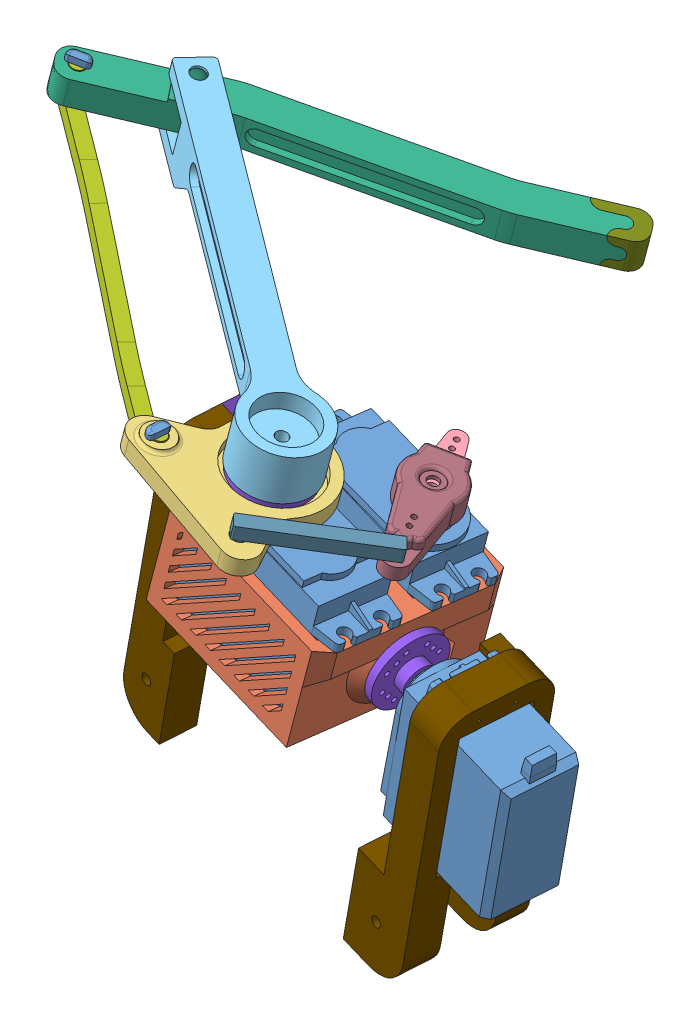
SolidWorks assembly Rear Robot Assembly, configuration Default. Lengths in mm.
Overall size (187.45 151.33 155.87).
34 component instances, 19 part files, 63 mates.
Components (placement in the parent):
- MG996R-1: MG996R [Default] at (29.5952 -122.5628 58.2658) x (-0.962615 0.249609 -0.105199) z (0.100626 -0.031047 -0.99444) size (54.5 42.75 20)
- MG996R-2: MG996R [Default] at (26.9789 -121.7556 84.1213) x (0.962615 -0.249609 0.105199) z (-0.100626 0.031047 0.99444) size (54.5 42.75 20)
- MG996R-3: MG996R [Default] at (100.7498 -138.2322 78.1733) x (-0.241344 -0.966685 -0.085287) z (0.122983 0.056709 -0.990787) size (54.5 42.75 20)
- Servo Housing-1: Servo Housing [Default] at (37.077 -93.7693 58.1239) x (-0.962615 0.249609 -0.105199) z (0.251487 0.967849 -0.00477) size (61.5 52 29.25)
- Rotating Piece-1: Rotating Piece [Default] at (26.8579 -80.6595 82.9278) x (0.452738 -0.121993 -0.883259) z (0.855443 -0.219969 0.468862) size (44.28 6 43.21)
- Double_Blade_Rudder-1: Double_Blade_Rudder [默认] at (51.0424 -81.5852 59.0548) x (0.86578 -0.227163 -0.445894) z (-0.432642 0.108008 -0.895073) size (12.2 5.5 38)
- Upper Leg-1: Upper Leg [Default] at (-58.4119 -49.1581 29.3225) x (-0.531201 0.142144 0.835237) z (0.251487 0.967849 -0.00477) size (22 116.4 18)
- Lower leg-1: Lower leg [Default] at (34.7159 -67.9253 -21.6894) x (0.593284 -0.150263 0.790845) z (-0.251487 -0.967849 0.00477) size (20.21 126 9.59)
- Long Connection Rod-1: Long Connection Rod [Default] at (10.1683 -76.252 97.3115) x (0.530048 -0.141848 -0.836019) z (-0.809817 0.20772 -0.548679) size (5 22 105.4)
- Circle Rudder-1: Circle Rudder [默认] at (57.8128 -116.2822 73.9977) x (0.107242 0.707834 0.698191) z (0.248738 0.660808 -0.70814) size (20.8 5.5 20.8)
- 688ZZ Bearing Assembly-2: 688ZZ Bearing Assembly [Default] at (1.0185 -101.5553 67.791) x (-0.264501 -0.949925 0.166376) z (-0.962615 0.249609 -0.105199) size (17.99 17.98 5)
  - Outer Ring-1: Outer Ring [Default] at origin size (16 16 5)
  - Inner Ring-1: Inner Ring [Default] x (-0.241565 -0.970385 0) z (0 0 1) size (10.6 10.6 5)
  - Cage-1: Cage [Default] x (0.535517 0.844524 0) z (0 0 1) size (13.01 13.06 2.21)
  - 2mm Ball Bearing-1: 2mm Ball Bearing [Default] at (-5.0671 3.2131 0) x (0.050652 0.835774 0.546732) z (0.977207 -0.154478 0.145614) size (2 2 2)
  - 2mm Ball Bearing-2: 2mm Ball Bearing [Default] at (-5.988 -0.3789 0) x (-0.450278 0.705928 0.546732) z (0.881377 0.449412 0.145614) size (2 2 2)
  - 2mm Ball Bearing-3: 2mm Ball Bearing [Default] at (-4.6217 -3.8262 0) x (-0.779216 0.306441 0.546732) z (0.448891 0.881642 0.145614) size (2 2 2)
  - 2mm Ball Bearing-4: 2mm Ball Bearing [Default] at (-1.49 -5.812 0) x (-0.810521 -0.210096 0.546732) z (-0.155056 0.977115 0.145614) size (2 2 2)
  - 2mm Ball Bearing-5: 2mm Ball Bearing [Default] at (2.2108 -5.5778 0) x (-0.532234 -0.646383 0.546732) z (-0.699777 0.699363 0.145614) size (2 2 2)
  - 2mm Ball Bearing-6: 2mm Ball Bearing [Default] at (5.0671 -3.2131 0) x (-0.050652 -0.835774 0.546732) z (-0.977207 0.154478 0.145614) size (2 2 2)
  - 2mm Ball Bearing-7: 2mm Ball Bearing [Default] at (5.988 0.3789 0) x (0.450278 -0.705928 0.546732) z (-0.881377 -0.449412 0.145614) size (2 2 2)
  - 2mm Ball Bearing-8: 2mm Ball Bearing [Default] at (4.6217 3.8262 0) x (0.779216 -0.306441 0.546732) z (-0.448891 -0.881642 0.145614) size (2 2 2)
  - 2mm Ball Bearing-9: 2mm Ball Bearing [Default] at (1.49 5.812 0) x (0.810521 0.210096 0.546732) z (0.155056 -0.977115 0.145614) size (2 2 2)
  - 2mm Ball Bearing-10: 2mm Ball Bearing [Default] at (-2.2108 5.5778 0) x (0.532234 0.646383 0.546732) z (0.699777 -0.699363 0.145614) size (2 2 2)
- Circle Rudder-3: Circle Rudder [默认] at (28.1908 -75.5299 82.9026) x (0.821577 -0.21087 0.529666) z (0.511631 -0.137123 -0.848193) size (20.8 5.5 20.8)
- Servo Arm Mount-1: Servo Arm Mount [Default] at (51.0424 -81.5852 59.0548) x (-0.86578 0.227163 0.445894) z (0.251487 0.967849 -0.00477) size (16.2 34.39 7.06)
- Short Connecting Rod-1: Short Connecting Rod [Default] at (63.207 -84.6449 79.6012) x (-0.679733 0.180127 0.710998) z (0.251487 0.967849 -0.00477) size (37.08 4 13)
- 91595A167_Dowel Pin-1: 91595A167_Dowel Pin [91595A167] at (-52.0367 -50.8228 27.674) x (-0.945505 0.244623 -0.214897) z (-0.251487 -0.967849 0.00477) size (4 4 20)
- Foot Cap-1: Foot Cap [Default] at (18.0805 -63.5858 -21.0299) x (0.593284 -0.150263 0.790845) z (-0.251487 -0.967849 0.00477) size (10.5 14 9.53)
- Lower Leg Mount-1: Lower Leg Mount [Default] at (-1.6759 -81.5579 68.6011) x (0.241344 0.966685 0.085287) z (0.962615 -0.249609 0.105199) size (41.75 15.4 10)
- Reverse Side Leg Mount-1: Reverse Side Leg Mount [Default] at (-136.4701 -136.4866 64.2689) x (0.241344 0.966685 0.085287) z (0.962615 -0.249609 0.105199) size (86 33.8 96.5)
- Rod Cap-1: Rod Cap [Default] at (-70.679 -41.0418 44.0662) x (-0.863943 0.226704 0.449674) z (0.436298 -0.108967 0.89318) size (6.08 7 3)
- Rod Cap-2: Rod Cap [Default] at (9.6296 -69.6975 99.0476) x (-0.054126 0.018984 0.998354) z (0.966346 -0.250815 0.05716) size (6.08 7 3)
- Rod Cap-3: Rod Cap [Default] at (35.666 -82.9502 103.5021) x (-0.679733 0.180127 0.710998) z (-0.688997 0.175565 -0.703178) size (6.08 7 3)
Mates (geometry in assembly coordinates):
- Coincident3: coincident aligned: plane of MG996R-1 through (49.2065 -88.6505 59.0896) normal (0.251487 0.967849 -0.00477); plane of MG996R-2 through (26.3549 -82.5952 82.9374) normal (0.251487 0.967849 -0.00477)
- Coincident4: coincident aligned: plane of MG996R-1 through (59.0851 -93.3273 50.2812) normal (0.962615 -0.249609 0.105199); plane of MG996R-2 through (54.4563 -91.8991 96.0254) normal (0.962615 -0.249609 0.105199)
- Distance1: distance = 6 mm anti-aligned: plane of MG996R-1 through (57.0726 -92.7063 70.17) normal (-0.100626 0.031047 0.99444); plane of MG996R-2 through (17.4829 -82.4109 71.8761) normal (0.100626 -0.031047 -0.99444)
- InPlace1: in place: plane of ? through (-38.4551 28.1284 17.4765) normal (0 1 0); plane of ? through (0 28.1284 0) normal (0 1 0); moOrthogonalPlaneRef_w of ? through (-38.4551 28.1284 17.4765) normal (0 1 0); plane of ? through (0 28.1284 0) normal (0 0 -1); plane of ? through (-38.4551 28.1284 17.4765) normal (0 1 0); plane of ? through (0 28.1284 0) normal (1 0 0); plane of MG996R-1 through (12.5314 -87.3809 60.2393) normal (0.251487 0.967849 -0.00477); unknown of Servo Housing-1
- Coincident6: coincident aligned: plane of MG996R-1; plane of Servo Housing-1
- Coincident7: coincident aligned: moOrthogonalPlaneRef_w of MG996R-1; plane of Servo Housing-1 through (37.077 -93.7693 58.1239) normal (-0.100626 0.031047 0.99444)
- Coincident8: coincident anti-aligned: moOrthogonalPlaneRef_w of MG996R-1; plane of Servo Housing-1 through (37.077 -93.7693 58.1239) normal (-0.962615 0.249609 -0.105199)
- Concentric1: concentric aligned: cylinder of MG996R-1 through (49.7095 -86.7148 59.0801) axis (0.251487 0.967849 -0.00477) radius 1.5; circle of Rotating Piece-1
- Coincident5: coincident anti-aligned: plane of MG996R-1 through (49.7095 -86.7148 59.0801) normal (0.251487 0.967849 -0.00477); plane of Rotating Piece-1 through (26.8579 -80.6595 82.9278) normal (-0.251487 -0.967849 0.00477)
- Coincident7: coincident anti-aligned: plane of MG996R-2 through (27.6124 -77.756 82.9135) normal (0.251487 0.967849 -0.00477); plane of Double_Blade_Rudder-1 through (50.4639 -83.8113 59.0657) normal (-0.251487 -0.967849 0.00477)
- Concentric2: concentric aligned: cylinder of MG996R-2 through (13.057 -90.8527 63.064) axis (0.25828 0.962853 -0.078774) radius 1.5; cylinder of Double_Blade_Rudder-1 through (36.5135 23.7673 6.6118) axis (0.25828 0.962853 -0.078774) radius 1.5
- Concentric3: concentric aligned: cylinder of Rotating Piece-1 through (27.3609 -78.7238 82.9183) axis (-0.251487 -0.967849 0.00477) radius 4.75; cylinder of Upper Leg-1 through (30.4542 -66.8193 82.8596) axis (-0.251487 -0.967849 0.00477) radius 1.5
- Concentric4: concentric aligned: cylinder of Upper Leg-1 through (-54.0486 -58.5656 27.7121) axis (0.251487 0.967849 -0.00477) radius 2.1; cylinder of Lower leg-1 through (-52.9169 -54.2102 27.6907) axis (0.251487 0.967849 -0.00477) radius 2
- Distance3: distance = 0.5 mm anti-aligned: plane of Lower leg-1 through (34.7159 -67.9253 -21.6894) normal (0.251487 0.967849 -0.00477); plane of Upper Leg-1 through (-48.4038 -45.6253 15.9301) normal (-0.251487 -0.967849 0.00477)
- LimitAngle3: limit planar angle = 1.561857 rad anti-aligned: plane of Lower leg-1 through (32.4525 -76.6359 -21.6465) normal (0.593284 -0.150263 0.790845); plane of Upper Leg-1 through (-50.585 -40.9011 20.9224) normal (0.531201 -0.142144 -0.835237)
- Coincident16: coincident anti-aligned: plane of Long Connection Rod-1 through (10.1683 -76.252 97.3115) normal (0.251487 0.967849 -0.00477); plane of Rotating Piece-1 through (26.8579 -80.6595 82.9278) normal (-0.251487 -0.967849 0.00477)
- Concentric9: concentric anti-aligned: cylinder of Lower leg-1 through (-47.0306 -55.7879 17.9084) axis (0.251487 0.967849 -0.00477) radius 2.1; cylinder of Connection Rod (temporary)-1 through (9.8786 -69.7627 98.9405) axis (-0.251487 -0.967849 0.00477) radius 2
- Coincident17: coincident anti-aligned: plane of Servo Housing-1 through (36.8825 -202.2704 61.4918) normal (0.962615 -0.249609 0.105199); plane of Circle Rudder-1 through (57.8128 -116.2822 73.9977) normal (-0.962615 0.249609 -0.105199)
- Concentric10: concentric aligned: circle of Servo Housing-1; circle of Circle Rudder-1
- Concentric11: concentric anti-aligned: cylinder of Servo Housing-1 through (-1.388 -100.9312 67.528) axis (0.962615 -0.249609 0.105199) radius 4; cylinder of 688ZZ Bearing Assembly-2/Inner Ring-1 through (-5.4843 -99.8691 67.0803) axis (-0.962615 0.249609 -0.105199) radius 4
- Coincident18: coincident aligned: plane of Servo Housing-1 through (4.1074 -85.2202 54.5209) normal (-0.962615 0.249609 -0.105199); plane of 688ZZ Bearing Assembly-2/Inner Ring-1 through (-2.6372 -105.9123 67.1397) normal (-0.962615 0.249609 -0.105199)
- Coincident19: coincident anti-aligned: plane of MG996R-1 through (50.4639 -83.8113 59.0657) normal (0.251487 0.967849 -0.00477); plane of Circle Rudder-3 through (27.6124 -77.756 82.9135) normal (-0.251487 -0.967849 0.00477)
- Coincident20: coincident anti-aligned: plane of Upper Leg-1 through (28.1908 -75.5299 82.9026) normal (-0.251487 -0.967849 0.00477); plane of Circle Rudder-3 through (28.1908 -75.5299 82.9026) normal (0.251487 0.967849 -0.00477)
- InPlace2: in place: plane of ? through (-72.3336 35.5583 10.554) normal (0 1 0); plane of ? through (0 35.5583 0) normal (0 1 0); plane of ? through (-72.3336 35.5583 10.554) normal (0 1 0); plane of ? through (0 35.5583 0) normal (0 0 -1); plane of ? through (-72.3336 35.5583 10.554) normal (0 1 0); plane of ? through (0 35.5583 0) normal (1 0 0); plane of Double_Blade_Rudder-1 through (51.0424 -81.5852 59.0548) normal (0.251487 0.967849 -0.00477); unknown of Servo Arm Mount-1
- Coincident21: coincident aligned: plane of Double_Blade_Rudder-1; plane of Servo Arm Mount-1
- Coincident22: coincident aligned: moOrthogonalPlaneRef_w of Double_Blade_Rudder-1; plane of Servo Arm Mount-1 through (51.0424 -81.5852 59.0548) normal (0.432642 -0.108008 0.895073)
- Coincident23: coincident anti-aligned: moOrthogonalPlaneRef_w of Double_Blade_Rudder-1; plane of Servo Arm Mount-1 through (51.0424 -81.5852 59.0548) normal (-0.86578 0.227163 0.445894)
- Concentric15: concentric anti-aligned: cylinder of Rotating Piece-1 through (37.9765 -78.2833 103.067) axis (-0.251487 -0.967849 0.00477) radius 2.2; cylinder of Short Connecting Rod-1 through (36.6939 -83.2193 103.0913) axis (0.251487 0.967849 -0.00477) radius 2
- Coincident24: coincident anti-aligned: plane of Short Connecting Rod-1 through (63.207 -84.6449 79.6012) normal (-0.251487 -0.967849 0.00477); plane of Servo Arm Mount-1 through (51.0424 -81.5852 59.0548) normal (0.251487 0.967849 -0.00477)
- Concentric16: concentric aligned: cylinder of Short Connecting Rod-1 through (59.4514 -89.2499 79.2871) axis (0.251487 0.967849 -0.00477) radius 1.5; cylinder of Servo Arm Mount-1 through (59.8035 -87.8949 79.2804) axis (0.251487 0.967849 -0.00477) radius 1.7
- Concentric18: concentric anti-aligned: cylinder of Upper Leg-1 through (-54.0486 -58.5656 27.7121) axis (0.251487 0.967849 -0.00477) radius 2.1; cylinder of 91595A167_Dowel Pin-1 through (-54.5516 -60.5013 27.7217) axis (-0.251487 -0.967849 0.00477) radius 2
- Tangent1: tangent aligned: sphere of 91595A167_Dowel Pin-1; plane of Upper Leg-1 through (-55.897 -39.4796 29.2748) normal (0.251487 0.967849 -0.00477)
- Concentric19: concentric aligned: cylinder of Lower leg-1 through (26.0295 -70.319 -21.9502) axis (0.593284 -0.150263 0.790845) radius 2; cylinder of Foot Cap-1 through (26.0295 -70.319 -21.9502) axis (0.593284 -0.150263 0.790845) radius 2
- Concentric22: concentric anti-aligned: cylinder of Lower leg-1 through (27.1612 -65.9636 -21.9717) axis (-0.251487 -0.967849 0.00477) radius 2; cylinder of Foot Cap-1 through (24.9012 -74.6614 -21.9288) axis (0.251487 0.967849 -0.00477) radius 2
- Coincident25: coincident: point of Foot Cap-1
- Tangent4: tangent aligned: cylinder of Foot Cap-1 through (-88.7667 -45.432 159.8118) axis (0.25828 0.962853 -0.078774) radius 4
- Concentric24: concentric aligned: cylinder of Circle Rudder-1 through (63.1072 -117.6551 74.5763) axis (-0.962615 0.249609 -0.105199) radius 3; cylinder of MG996R-3 through (65.0324 -118.1543 74.7867) axis (-0.962615 0.249609 -0.105199) radius 1.5
- Concentric25: concentric anti-aligned: cylinder of 688ZZ Bearing Assembly-2/Outer Ring-1 through (-5.4843 -99.8691 67.0803) axis (-0.962615 0.249609 -0.105199) radius 8; cylinder of Reverse Side Leg Mount-1 through (-6.2011 -99.6832 67.002) axis (0.962615 -0.249609 0.105199) radius 8
- Coincident26: coincident aligned: plane of 688ZZ Bearing Assembly-2/Outer Ring-1 through (3.0162 -100.8634 74.917) normal (0.962615 -0.249609 0.105199); plane of Reverse Side Leg Mount-1 through (18.6005 -79.1429 -16.1491) normal (0.962615 -0.249609 0.105199)
- Coincident27: coincident anti-aligned: plane of MG996R-3 through (79.9653 -107.5338 82.1666) normal (0.962615 -0.249609 0.105199); plane of Reverse Side Leg Mount-1 through (92.2406 -98.238 -8.1013) normal (-0.962615 0.249609 -0.105199)
- Parallel1: parallel anti-aligned: plane of MG996R-3 through (69.9937 -110.3004 86.0473) normal (-0.122983 -0.056709 0.990787); plane of Reverse Side Leg Mount-1 through (88.2982 -112.9793 88.0638) normal (0.122983 0.056709 -0.990787)
- Coincident29: coincident anti-aligned: plane of Lower Leg Mount-1 through (1.4943 -109.9128 67.3717) normal (-0.122983 -0.056709 0.990787); plane of Reverse Side Leg Mount-1 through (1.4943 -109.9128 67.3717) normal (0.122983 0.056709 -0.990787)
- Coincident30: coincident anti-aligned: plane of Lower Leg Mount-1 through (-2.1259 -124.413 66.0924) normal (-0.241344 -0.966685 -0.085287); plane of Reverse Side Leg Mount-1 through (-2.1259 -124.413 66.0924) normal (0.241344 0.966685 0.085287)
- Coincident31: coincident aligned: plane of Lower Leg Mount-1 through (-6.2011 -99.6832 67.002) normal (-0.962615 0.249609 -0.105199); plane of Reverse Side Leg Mount-1 through (-24.3254 -165.5661 76.5246) normal (-0.962615 0.249609 -0.105199)
- Concentric28: concentric aligned: cylinder of MG996R-2 through (26.8579 -80.6595 82.9278) axis (0.251487 0.967849 -0.00477) radius 1.5; cylinder of Circle Rudder-3 through (27.6124 -77.756 82.9135) axis (0.251487 0.967849 -0.00477) radius 1.5
- Coincident32: coincident anti-aligned: plane of MG996R-2 through (27.6124 -77.756 82.9135) normal (0.251487 0.967849 -0.00477); plane of Circle Rudder-3 through (27.6124 -77.756 82.9135) normal (-0.251487 -0.967849 0.00477)
- Coincident33: coincident anti-aligned: plane of Upper Leg-1 through (28.1908 -75.5299 82.9026) normal (-0.251487 -0.967849 0.00477); plane of Circle Rudder-3 through (28.1908 -75.5299 82.9026) normal (0.251487 0.967849 -0.00477)
- Concentric29: concentric anti-aligned: cylinder of Upper Leg-1 through (30.4542 -66.8193 82.8596) axis (-0.251487 -0.967849 0.00477) radius 1.7; cylinder of Circle Rudder-3 through (27.6124 -77.756 82.9135) axis (0.251487 0.967849 -0.00477) radius 1.5
- Concentric30: concentric anti-aligned: cylinder of Rotating Piece-1 through (27.3609 -78.7238 82.9183) axis (-0.251487 -0.967849 0.00477) radius 4.5; cylinder of Circle Rudder-3 through (26.8076 -80.8531 82.9288) axis (0.251487 0.967849 -0.00477) radius 4.4
- Coincident34: coincident anti-aligned: plane of MG996R-2 through (26.8579 -80.6595 82.9278) normal (0.251487 0.967849 -0.00477); plane of Rotating Piece-1 through (26.8579 -80.6595 82.9278) normal (-0.251487 -0.967849 0.00477)
- Concentric31: concentric aligned: cylinder of MG996R-1 through (49.7095 -86.7148 59.0801) axis (0.251487 0.967849 -0.00477) radius 1.5; cylinder of Double_Blade_Rudder-1 through (49.6592 -86.9084 59.081) axis (0.251487 0.967849 -0.00477) radius 3
- Coincident35: coincident anti-aligned: plane of MG996R-1 through (50.4639 -83.8113 59.0657) normal (0.251487 0.967849 -0.00477); plane of Double_Blade_Rudder-1 through (50.4639 -83.8113 59.0657) normal (-0.251487 -0.967849 0.00477)
- Concentric33: concentric aligned: cylinder of Rotating Piece-1 through (8.7461 -70.7136 97.8624) axis (-0.251487 -0.967849 0.00477) radius 2.2; cylinder of Long Connection Rod-1 through (9.0478 -69.5522 97.8567) axis (-0.251487 -0.967849 0.00477) radius 2
- Concentric35: concentric anti-aligned: cylinder of Lower leg-1 through (-72.0345 -49.1673 42.9906) axis (0.251487 0.967849 -0.00477) radius 2.1; cylinder of Long Connection Rod-1 through (-69.9723 -41.2309 42.9515) axis (-0.251487 -0.967849 0.00477) radius 2
- Coincident36: coincident anti-aligned: plane of Long Connection Rod-1 through (-70.4442 -48.3403 43.0611) normal (-0.436298 0.108967 -0.89318); plane of Rod Cap-1 through (-71.9364 -45.8811 44.0901) normal (0.436298 -0.108967 0.89318)
- Coincident37: coincident anti-aligned: plane of Long Connection Rod-1 through (-72.4394 -47.8168 44.0996) normal (0.966346 -0.250815 0.05716); plane of Rod Cap-1 through (-71.8239 -45.9205 42.015) normal (-0.966346 0.250815 -0.05716)
- Coincident38: coincident anti-aligned: plane of Long Connection Rod-1 through (-69.9723 -41.2309 42.9515) normal (0.251487 0.967849 -0.00477); plane of Rod Cap-1 through (-71.1153 -40.9328 43.1731) normal (-0.251487 -0.967849 0.00477)
- Coincident39: coincident anti-aligned: plane of Long Connection Rod-1 through (7.8692 -76.4724 99.0809) normal (0.530048 -0.141848 -0.836019); plane of Rod Cap-2 through (6.689 -74.105 97.931) normal (-0.530048 0.141848 0.836019)
- Coincident40: coincident anti-aligned: plane of Long Connection Rod-1 through (7.9942 -76.5163 96.7753) normal (-0.966346 0.250815 -0.05716); plane of Rod Cap-2 through (8.3721 -74.5367 99.0714) normal (0.966346 -0.250815 0.05716)
- Coincident41: coincident anti-aligned: plane of Long Connection Rod-1 through (9.0478 -69.5522 97.8567) normal (0.251487 0.967849 -0.00477); plane of Rod Cap-2 through (8.6632 -69.4467 98.9904) normal (-0.251487 -0.967849 0.00477)
- Coincident42: coincident anti-aligned: plane of Short Connecting Rod-1 through (54.5337 -87.8276 108.6085) normal (0.244167 -0.068212 -0.967331); plane of Rod Cap-3 through (38.87 -78.6141 104.0051) normal (-0.244167 0.068212 0.967331)
- Coincident43: coincident anti-aligned: plane of Short Connecting Rod-1 through (33.269 -82.4051 87.7172) normal (-0.933165 0.243777 0.264153); plane of Rod Cap-3 through (38.3362 -78.4853 102.0004) normal (0.933165 -0.243777 -0.264153)
- Coincident44: coincident anti-aligned: plane of Short Connecting Rod-1 through (61.849 -89.8713 79.627) normal (-0.251487 -0.967849 0.00477); plane of Rod Cap-3 through (36.355 -83.1257 104.2052) normal (0.251487 0.967849 -0.00477)
